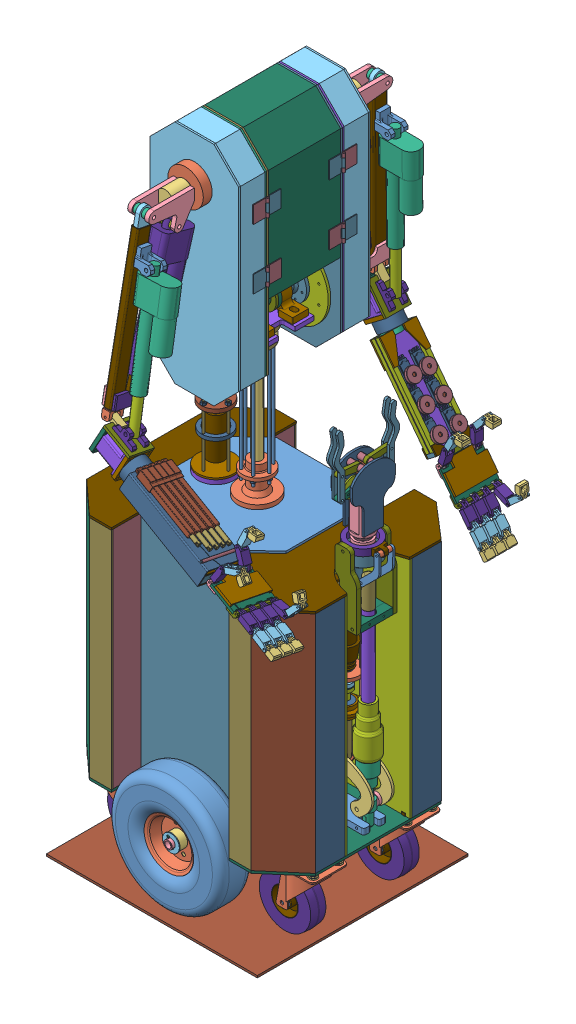
SolidWorks assembly sorbot, configuration По умолчанию. Lengths in mm. (continued)
Mates (geometry in assembly coordinates): (continued)
- Концентричный339: concentric aligned: cylinder of palm.fixture.p13-1 through (365.6621 758.5087 201.9382) axis (-0.001246 0.191494 0.981493) radius 1.5; cylinder of finger.p1-2 through (365.6602 758.8068 203.466) axis (-0.001246 0.191494 0.981493) radius 1.5
- Концентричный342: concentric aligned: cylinder of palm.fixture.p13-1 through (365.6621 758.5087 201.9382) axis (-0.001246 0.191494 0.981493) radius 1.5; cylinder of finger.p1-3 through (365.5966 768.573 253.5221) axis (-0.001246 0.191494 0.981493) radius 1.5
- Параллельность165: parallel aligned: plane of palm.p1-3 through (361.7576 760.7842 201.5469) normal (0.410922 0.894897 -0.174077); plane of finger.p1-3 through (409.4727 760.6234 276.0154) normal (0.410922 0.894897 -0.174077)
- Совпадение637: coincident anti-aligned: plane of palm.p1-3 through (359.2921 755.4149 202.5914) normal (-0.410922 -0.894897 0.174077); plane of palm.p3.m-1 through (320.3506 791.7274 297.3428) normal (0.410922 0.894897 -0.174077)
- Совпадение638: coincident aligned: plane of palm.p1-3 through (293.2577 810.1661 293.7109) normal (-0.001246 0.191494 0.981493); plane of palm.p3.m-1 through (294.9764 811.5594 293.4412) normal (-0.001246 0.191494 0.981493)
- Совпадение640: coincident anti-aligned: plane of palm.p3.m-1 through (303.6145 808.8356 293.9836) normal (0.91167 -0.4031 0.079805); plane of palm.p1-3 through (302.4043 801.5393 270.9531) normal (-0.91167 0.4031 -0.079805)
- Совпадение641: coincident anti-aligned: plane of palm.p3-1 through (354.922 753.9955 207.957) normal (-0.001246 0.191494 0.981493); plane of finger.p1-2 through (353.8618 756.4881 207.4694) normal (0.001246 -0.191494 -0.981493)
- Концентричный345: concentric aligned: cylinder of palm.fixture.p13-1 through (365.6621 758.5087 201.9382) axis (-0.001246 0.191494 0.981493) radius 1.5; cylinder of finger.p1-4 through (365.6284 763.6899 228.494) axis (-0.001246 0.191494 0.981493) radius 1.5
- Параллельность167: parallel aligned: plane of palm.p1-3 through (361.7576 760.7842 201.5469) normal (0.410922 0.894897 -0.174077); plane of finger.p1-4 through (409.5045 755.7403 250.9873) normal (0.410922 0.894897 -0.174077)
- Совпадение645: coincident anti-aligned: plane of palm.p1-3 through (359.2921 755.4149 202.5914) normal (-0.410922 -0.894897 0.174077); plane of palm.p3.m-2 through (320.4484 776.6951 220.2956) normal (0.410922 0.894897 -0.174077)
- Совпадение646: coincident aligned: plane of palm.p1-3 through (293.3824 791.0167 195.5616) normal (0.001246 -0.191494 -0.981493); plane of palm.p3.m-2 through (295.1011 792.41 195.2919) normal (0.001246 -0.191494 -0.981493)
- Совпадение647: coincident anti-aligned: plane of palm.p3.m-2 through (303.7123 793.8034 216.9364) normal (0.91167 -0.4031 0.079805); plane of palm.p1-3 through (302.4692 791.5816 219.9154) normal (-0.91167 0.4031 -0.079805)
- Заблокировать267: lock: unknown of ?; unknown of ?
- Концентричный348: concentric aligned: cylinder of palm.p3.m-1 through (297.351 805.9631 294.5361) axis (0.001246 -0.191494 -0.981493) radius 1.5; cylinder of finger.p1-5 through (297.3517 805.8673 294.0454) axis (0.001246 -0.191494 -0.981493) radius 1.5
- Совпадение648: coincident anti-aligned: plane of palm.p3.m-1 through (284.5507 802.4864 291.1227) normal (0.001246 -0.191494 -0.981493); plane of finger.p1-5 through (287.412 798.2914 291.9448) normal (-0.001246 0.191494 0.981493)
- Концентричный351: concentric aligned: cylinder of finger.p1-6 through (297.4494 790.8542 217.0963) axis (0.001246 -0.191494 -0.981493) radius 1.5; cylinder of palm.p3.m-2 through (297.4489 790.9308 217.4889) axis (0.001246 -0.191494 -0.981493) radius 1.5
- Концентричный352: concentric aligned: cylinder of finger.p1-1 through (402.282 756.6831 281.8693) axis (-0.001246 0.191494 0.981493) radius 1.5; cylinder of finger.p2-7 through (402.282 756.6831 281.8693) axis (-0.001246 0.191494 0.981493) radius 1.5
- Совпадение652: coincident anti-aligned: plane of finger.p1-1 through (393.5748 758.839 298.2487) normal (0.001246 -0.191494 -0.981493); plane of finger.p2-7 through (390.7532 760.3857 297.9434) normal (-0.001246 0.191494 0.981493)
- Концентричный354: concentric aligned: cylinder of finger.p3-1 through (437.4075 740.08 285.2682) axis (-0.001246 0.191494 0.981493) radius 1.5; cylinder of finger.p2-7 through (437.4076 740.0584 285.1575) axis (-0.001246 0.191494 0.981493) radius 1.5
- Совпадение653: coincident: plane of ? through (235.2448 521.1837 179.8569) normal (0.004463 0.000114 0.99999); plane of ? through (237.0318 518.7761 179.8492) normal (-0.004463 -0.000114 -0.99999)
- Концентричный355: concentric aligned: cylinder of finger.p1-3 through (402.3138 751.8 256.8412) axis (-0.001246 0.191494 0.981493) radius 1.5; cylinder of finger.p2-8 through (402.3138 751.8 256.8412) axis (-0.001246 0.191494 0.981493) radius 1.5
- Совпадение654: coincident anti-aligned: plane of finger.p1-3 through (393.6066 753.9559 273.2207) normal (0.001246 -0.191494 -0.981493); plane of finger.p2-8 through (390.7757 755.2583 272.963) normal (-0.001246 0.191494 0.981493)
- Концентричный356: concentric aligned: cylinder of finger.p1-4 through (402.3456 746.9169 231.8131) axis (-0.001246 0.191494 0.981493) radius 1.5; cylinder of finger.p2-9 through (402.3456 746.9169 231.8131) axis (-0.001246 0.191494 0.981493) radius 1.5
- Совпадение655: coincident anti-aligned: plane of finger.p1-4 through (393.6383 749.0728 248.1926) normal (0.001246 -0.191494 -0.981493); plane of finger.p2-9 through (390.8061 750.3187 247.9459) normal (-0.001246 0.191494 0.981493)
- Концентричный357: concentric aligned: cylinder of finger.p1-2 through (405.4877 751.586 204.9254) axis (-0.001246 0.191494 0.981493) radius 1.5; cylinder of finger.p2-10 through (405.4877 751.586 204.9254) axis (-0.001246 0.191494 0.981493) radius 1.5
- Совпадение656: coincident anti-aligned: plane of finger.p1-2 through (397.3122 751.6404 221.7155) normal (0.001246 -0.191494 -0.981493); plane of finger.p2-10 through (401.7717 744.0338 223.2052) normal (-0.001246 0.191494 0.981493)
- Концентричный358: concentric aligned: cylinder of finger.p3-2 through (431.4304 780.1948 199.4916) axis (-0.001246 0.191494 0.981493) radius 1.5; cylinder of finger.p2-10 through (431.4305 780.1732 199.3808) axis (-0.001246 0.191494 0.981493) radius 1.5
- Совпадение657: coincident anti-aligned: plane of finger.p3-2 through (439.6172 775.3981 217.134) normal (-0.001246 0.191494 0.981493); plane of finger.p2-10 through (429.781 774.8981 217.219) normal (0.001246 -0.191494 -0.981493)
- Концентричный359: concentric aligned: cylinder of finger.p1-5 through (317.4709 840.3743 287.3384) axis (0.001246 -0.191494 -0.981493) radius 1.5; cylinder of finger.p2-11 through (317.4709 840.3743 287.3384) axis (0.001246 -0.191494 -0.981493) radius 1.5
- Совпадение658: coincident anti-aligned: plane of finger.p1-5 through (309.7926 835.5044 284.2034) normal (0.001246 -0.191494 -0.981493); plane of finger.p2-11 through (306.0326 840.9226 283.1415) normal (-0.001246 0.191494 0.981493)
- Концентричный360: concentric aligned: cylinder of finger.p3-5 through (354.9027 851.1497 285.3986) axis (0.001246 -0.191494 -0.981493) radius 1.5; cylinder of finger.p2-11 through (354.9028 851.1281 285.2878) axis (0.001246 -0.191494 -0.981493) radius 1.5
- Совпадение659: coincident anti-aligned: plane of finger.p3-5 through (352.0131 861.3071 279.2228) normal (-0.001246 0.191494 0.981493); plane of finger.p2-11 through (346.4462 852.5329 280.9276) normal (0.001246 -0.191494 -0.981493)
- Концентричный362: concentric aligned: cylinder of finger.p1-6 through (278.3051 825.8821 210.2379) axis (0.001246 -0.191494 -0.981493) radius 1.5; cylinder of finger.p2-12 through (278.3051 825.8821 210.2379) axis (0.001246 -0.191494 -0.981493) radius 1.5
- Совпадение661: coincident anti-aligned: plane of finger.p1-6 through (277.7816 816.5471 207.9831) normal (0.001246 -0.191494 -0.981493); plane of finger.p2-12 through (270.3574 816.9317 207.8986) normal (-0.001246 0.191494 0.981493)
- Концентричный363: concentric aligned: cylinder of ? through (195.7839 707.1121 106.7239) axis (-0.004463 -0.000114 -0.99999) radius 1.5; cylinder of ? through (195.7834 707.1121 106.6111) axis (-0.004463 -0.000114 -0.99999) radius 1.5
- Совпадение662: coincident: plane of ? through (190.3026 717.2558 102.6343) normal (0.004463 0.000114 0.99999); plane of ? through (187.0589 706.2794 102.6501) normal (-0.004463 -0.000114 -0.99999)
- Совпадение664: coincident anti-aligned: plane of palm.p3-1 through (365.7816 761.5097 272.221) normal (0.001246 -0.191494 -0.981493); plane of finger.p1-3 through (353.3954 771.831 270.1915) normal (-0.001246 0.191494 0.981493)
- Совпадение665: coincident anti-aligned: plane of palm.p3-1 through (365.8134 756.6266 247.1929) normal (0.001246 -0.191494 -0.981493); plane of finger.p1-4 through (353.4271 766.9479 245.1634) normal (-0.001246 0.191494 0.981493)
- Совпадение666: coincident anti-aligned: plane of palm.p1-3 through (361.7576 760.7842 201.5469) normal (0.410922 0.894897 -0.174077); plane of palm.p5-1 through (331.4609 789.3117 276.6833) normal (-0.410922 -0.894897 0.174077)
- Совпадение667: coincident anti-aligned: plane of palm.p1-3 through (361.7576 760.7842 201.5469) normal (0.410922 0.894897 -0.174077); plane of palm.p6-1 through (302.9044 799.3879 261.0737) normal (-0.410922 -0.894897 0.174077)
- Совпадение668: coincident anti-aligned: plane of palm.p1-3 through (361.7576 760.7842 201.5469) normal (0.410922 0.894897 -0.174077); plane of palm.p5-2 through (331.5169 778.2186 219.7881) normal (-0.410922 -0.894897 0.174077)
- Совпадение669: coincident anti-aligned: plane of palm.p1-3 through (361.7576 760.7842 201.5469) normal (0.410922 0.894897 -0.174077); plane of palm.p6-2 through (302.8729 793.2734 229.5656) normal (-0.410922 -0.894897 0.174077)
- Заблокировать268: lock: unknown of ?; unknown of ?
- Заблокировать269: lock: unknown of ?; unknown of ?
- Концентричный367: concentric anti-aligned: cylinder of finger.actuator.p2-5 through (240.3211 845.5977 266.3536) axis (-0.91167 0.4031 -0.079805) radius 4.5; cylinder of finger.actuator.p1-3 through (128.7399 894.9339 256.5862) axis (0.91167 -0.4031 0.079805) radius 4.5
- Параллельность169: parallel anti-aligned: cylinder of finger.actuator.p1-3 through (90.9006 912.4285 257.2003) axis (0.001246 -0.191494 -0.981493) radius 2.1; cylinder of finger.actuator.p2-5 through (243.9733 843.1236 262.2561) axis (-0.001246 0.191494 0.981493) radius 2.1
- Концентричный368: concentric anti-aligned: cylinder of finger.actuator.p1-4 through (128.7773 889.1891 227.1414) axis (0.91167 -0.4031 0.079805) radius 4.5; cylinder of finger.actuator.p2-6 through (255.2287 833.2779 238.2105) axis (-0.91167 0.4031 -0.079805) radius 4.5
- Параллельность171: parallel anti-aligned: cylinder of finger.actuator.p1-4 through (90.938 906.6837 227.7555) axis (0.001246 -0.191494 -0.981493) radius 2.1; cylinder of finger.actuator.p2-6 through (258.881 830.8038 234.113) axis (-0.001246 0.191494 0.981493) radius 2.1
- Концентричный370: concentric anti-aligned: cylinder of finger.actuator.p1-5 through (128.7586 892.0615 241.8638) axis (0.91167 -0.4031 0.079805) radius 4.5; cylinder of finger.actuator.p2-7 through (254.035 836.6698 252.8301) axis (-0.91167 0.4031 -0.079805) radius 4.5
- Параллельность173: parallel anti-aligned: cylinder of finger.actuator.p1-5 through (90.9193 909.5561 242.4779) axis (0.001246 -0.191494 -0.981493) radius 2.1; cylinder of finger.actuator.p2-7 through (257.6873 834.1957 248.7326) axis (-0.001246 0.191494 0.981493) radius 2.1
- Концентричный371: concentric anti-aligned: cylinder of finger.actuator.p1-6 through (128.8147 883.4443 197.6966) axis (0.91167 -0.4031 0.079805) radius 4.5; cylinder of finger.actuator.p2-8 through (255.925 827.2418 208.8234) axis (-0.91167 0.4031 -0.079805) radius 4.5
- Параллельность175: parallel anti-aligned: cylinder of finger.actuator.p1-6 through (90.9754 900.9389 198.3107) axis (0.001246 -0.191494 -0.981493) radius 2.1; cylinder of finger.actuator.p2-8 through (259.5773 824.7676 204.7259) axis (-0.001246 0.191494 0.981493) radius 2.1
- Концентричный372: concentric anti-aligned: cylinder of finger.actuator.p1-7 through (128.796 886.3167 212.419) axis (0.91167 -0.4031 0.079805) radius 4.5; cylinder of ? through (255.6249 830.2386 223.5212) axis (-0.91167 0.4031 -0.079805) radius 4.5
- Параллельность177: parallel anti-aligned: cylinder of finger.actuator.p1-7 through (90.9567 903.8113 213.0331) axis (0.001246 -0.191494 -0.981493) radius 2.1; cylinder of ? through (259.2772 827.7644 219.4237) axis (-0.001246 0.191494 0.981493) radius 2.1
- Заблокировать270: lock: unknown of ?; unknown of ?
- Заблокировать271: lock: unknown of ?; unknown of ?
- Совпадение675: coincident anti-aligned: plane of arm.cap-1 through (83.1026 909.5205 266.9275) normal (0.410922 0.894897 -0.174077); plane of finger.actuator.p1-5 through (125.6674 886.786 250.5306) normal (-0.410922 -0.894897 0.174077)
- Совпадение676: coincident anti-aligned: plane of arm.cap-1 through (83.1026 909.5205 266.9275) normal (0.410922 0.894897 -0.174077); plane of finger.actuator.p1-7 through (125.7048 881.0411 221.0858) normal (-0.410922 -0.894897 0.174077)
- Совпадение677: coincident anti-aligned: plane of arm.cap-1 through (83.1026 909.5205 266.9275) normal (0.410922 0.894897 -0.174077); plane of finger.actuator.p1-4 through (125.6861 883.9136 235.8082) normal (-0.410922 -0.894897 0.174077)
- Совпадение678: coincident anti-aligned: plane of arm.cap-1 through (83.1026 909.5205 266.9275) normal (0.410922 0.894897 -0.174077); plane of finger.actuator.p1-6 through (125.7235 878.1687 206.3634) normal (-0.410922 -0.894897 0.174077)
- Заблокировать272: lock: unknown of ?; unknown of ?
- Заблокировать273: lock: unknown of ?; unknown of ?
- Заблокировать274: lock: unknown of ?; unknown of ?
- Концентричный373: concentric aligned: cylinder of finger.actuator.p1-3 through (90.9006 912.4285 257.2003) axis (0.001246 -0.191494 -0.981493) radius 2.1; cylinder of finger.actuator.p1-5 through (90.9193 909.5561 242.4779) axis (0.001246 -0.191494 -0.981493) radius 2.1
- Концентричный374: concentric aligned: cylinder of finger.actuator.p1-3 through (90.9006 912.4285 257.2003) axis (0.001246 -0.191494 -0.981493) radius 2.1; cylinder of finger.actuator.p1-4 through (90.938 906.6837 227.7555) axis (0.001246 -0.191494 -0.981493) radius 2.1
- Концентричный375: concentric aligned: cylinder of finger.actuator.p1-3 through (90.9006 912.4285 257.2003) axis (0.001246 -0.191494 -0.981493) radius 2.1; cylinder of finger.actuator.p1-7 through (90.9567 903.8113 213.0331) axis (0.001246 -0.191494 -0.981493) radius 2.1
- Концентричный376: concentric aligned: cylinder of finger.actuator.p1-3 through (90.9006 912.4285 257.2003) axis (0.001246 -0.191494 -0.981493) radius 2.1; cylinder of finger.actuator.p1-6 through (90.9754 900.9389 198.3107) axis (0.001246 -0.191494 -0.981493) radius 2.1
- Совпадение680: coincident anti-aligned: plane of finger.actuator.p1-3 through (131.8312 900.2094 247.9194) normal (0.001246 -0.191494 -0.981493); plane of finger.actuator.p1-5 through (131.8312 900.2094 247.9194) normal (-0.001246 0.191494 0.981493)
- Совпадение681: coincident anti-aligned: plane of finger.actuator.p1-4 through (131.8499 897.337 233.197) normal (-0.001246 0.191494 0.981493); plane of finger.actuator.p1-5 through (131.8499 897.337 233.197) normal (0.001246 -0.191494 -0.981493)
- Совпадение682: coincident anti-aligned: plane of finger.actuator.p1-4 through (131.8686 894.4646 218.4746) normal (0.001246 -0.191494 -0.981493); plane of finger.actuator.p1-7 through (131.8686 894.4646 218.4746) normal (-0.001246 0.191494 0.981493)
- Совпадение683: coincident anti-aligned: plane of finger.actuator.p1-6 through (131.8873 891.5922 203.7522) normal (-0.001246 0.191494 0.981493); plane of finger.actuator.p1-7 through (131.8873 891.5922 203.7522) normal (0.001246 -0.191494 -0.981493)
- Заблокировать275: lock: unknown of ?; unknown of ?
- Заблокировать276: lock: unknown of ?; unknown of ?
- Заблокировать277: lock: unknown of ?; unknown of ?
- Заблокировать278: lock: unknown of ?; unknown of ?
- Заблокировать279: lock: unknown of ?; unknown of ?
- Концентричный378: concentric aligned: cylinder of fingers.fixture.p2-2 through (272.0168 832.2235 287.0411) axis (0.001246 -0.191494 -0.981493) radius 2; cylinder of fingers.fixture.p1-2 through (272.014 832.6632 289.2946) axis (0.001246 -0.191494 -0.981493) radius 1.75
- Совпадение690: coincident anti-aligned: plane of lower.arm.p8-2 through (267.6618 778.8108 292.664) normal (0.91167 -0.4031 0.079805); plane of palm.fixture.p14-1 through (271.2358 781.1563 263.6829) normal (-0.91167 0.4031 -0.079805)
- Совпадение692: coincident anti-aligned: plane of arm.p1.m-1 through (-3.763 974.0415 223.4385) normal (1 0 0); plane of forearm.rotate.p12-m-1 through (-3.763 994.3192 220.6386) normal (-1 0 0)
- Параллельность178: parallel aligned: plane of forearm.rotate.p12-m-1 through (-3.763 974.256 224.5414) normal (0 0.190943 0.981601); plane of arm.p1.m-1 through (-18.263 974.7098 226.8741) normal (0 0.190943 0.981601)
- Заблокировать282: lock: unknown of ?; unknown of ?
- Совпадение696: coincident anti-aligned: plane of ? through (5.2041 922.3385 146.0785) normal (-0.840373 -0.541996 0.003813); plane of ? through (35.0967 876.1313 166.2278) normal (0.840373 0.541996 -0.003813)
- Заблокировать283: lock: unknown of ?; unknown of ?
- Заблокировать284: lock: unknown of ?; unknown of ?
- Заблокировать286: lock: unknown of ?; unknown of ?
- Концентричный381: concentric aligned: cylinder of finger.p3-3 through (437.7973 735.9485 260.107) axis (-0.001246 0.191494 0.981493) radius 1.5; cylinder of finger.p2-8 through (437.7975 735.9245 259.9837) axis (-0.001246 0.191494 0.981493) radius 1.5
- Концентричный382: concentric aligned: cylinder of finger.p3-4 through (437.9098 731.2007 234.8449) axis (-0.001246 0.191494 0.981493) radius 1.5; cylinder of finger.p2-9 through (437.9097 731.2157 234.9217) axis (-0.001246 0.191494 0.981493) radius 1.5
- Заблокировать287: lock: unknown of ?; unknown of ?
- Заблокировать288: lock: unknown of ?; unknown of ?
- Заблокировать289: lock: unknown of ?; unknown of ?
- Заблокировать290: lock: unknown of ?; unknown of ?
- Заблокировать291: lock: unknown of ?; unknown of ?
- Заблокировать293: lock: unknown of ?; unknown of ?
- Заблокировать294: lock: unknown of ?; unknown of ?
- Заблокировать295: lock: unknown of ?; unknown of ?
- Заблокировать296: lock: unknown of ?; unknown of ?
- Заблокировать297: lock: unknown of ?; unknown of ?
- Заблокировать298: lock: unknown of ?; unknown of ?
- Заблокировать299: lock: unknown of ?; unknown of ?
- Заблокировать301: lock: unknown of ?; unknown of ?
- Заблокировать302: lock: unknown of ?; unknown of ?
- Заблокировать304: lock: unknown of ?; unknown of ?
- Заблокировать305: lock: unknown of ?; unknown of ?
- Заблокировать306: lock: unknown of ?; unknown of ?
- Заблокировать307: lock: unknown of ?; unknown of ?
- Заблокировать308: lock: unknown of ?; unknown of ?
- Заблокировать309: lock: unknown of ?; unknown of ?
- Заблокировать310: lock: unknown of ?; unknown of ?
- Заблокировать311: lock: unknown of ?; unknown of ?
- Заблокировать313: lock: unknown of ?; unknown of ?
- Концентричный385: concentric aligned: cylinder of forearm.rotate.p9-1 through (-12.6985 951.7393 197.5021) axis (0 0.190943 0.981601) radius 2.5; cylinder of forearm.rotate.p10-1 through (-12.6985 953.4041 206.0607) axis (0 0.190943 0.981601) radius 2.5
- Заблокировать314: lock: unknown of ?; unknown of ?
- Заблокировать315: lock: unknown of ?; unknown of ?
- Заблокировать316: lock: unknown of ?; unknown of ?
- Заблокировать317: lock: unknown of ?; unknown of ?
- Заблокировать318: lock: unknown of ?; unknown of ?
- Совпадение698: coincident anti-aligned: plane of forearm.rotate.p7-1 through (65.0333 926.3354 250.3973) normal (0.410922 0.894897 -0.174077); plane of forearm.rotate.p8-1 through (58.959 925.2061 230.253) normal (-0.410922 -0.894897 0.174077)
- Совпадение699: coincident anti-aligned: plane of forearm.rotate.p7-1 through (65.0333 926.3354 250.3973) normal (0.410922 0.894897 -0.174077); plane of forearm.rotate.p8-2 through (58.959 919.4778 200.805) normal (-0.410922 -0.894897 0.174077)
- Заблокировать319: lock: unknown of ?; unknown of ?
- Концентричный386: concentric aligned: cylinder of body.frame.p1-3 through (-12.4559 1335.4922 -50.7442) axis (0 0 1) radius 43; cylinder of arm.fixture.cap-1 through (-12.4559 1335.4922 -73.2442) axis (0 0 1) radius 45
- Заблокировать330: lock: unknown of ?; unknown of ?
- Заблокировать336: lock: unknown of ?; unknown of ?
- Заблокировать337: lock: unknown of ?; unknown of ?
- Заблокировать344: lock: unknown of body_tilt_drive_frame_cap-1; unknown of ?
- Заблокировать351: lock: unknown of turret.table.cap-1; unknown of body_tilt_drive_frame_cap-1
- Совпадение740: coincident anti-aligned: plane of shoulder.bearing.housing-2 through (-12.4903 1335.516 -46.7442) normal (0 0 1); plane of body.frame.p4.right-1 through (-117.4903 1436.2936 -46.7442) normal (0 0 -1)
- Концентричный404: concentric aligned: cylinder of shoulder.bearing.housing-1 through (-12.7629 1335.3853 40.2558) axis (0 0 -1) radius 15.5; cylinder of ? through (-12.7629 1335.3853 44.2558) axis (0 0 -1) radius 15
- Совпадение742: coincident: unknown of ?; unknown of ?
- Заблокировать361: lock: unknown of ?; unknown of ?
- Заблокировать362: lock: unknown of ?; unknown of ?
- Совпадение745: coincident anti-aligned: plane of body.frame.p5-1 through (92.4017 957.5916 592.5032) normal (1 0 0); plane of cap-hinge-1 through (92.4017 1325.4557 -46.5922) normal (-1 0 0)
- Совпадение746: coincident anti-aligned: plane of body.frame.p5-1 through (92.4017 957.5916 592.5032) normal (1 0 0); plane of cap-hinge-p1-2 through (92.4017 1182.6154 -46.8053) normal (-1 0 0)
- Концентричный405: concentric anti-aligned: cylinder of cap-hinge-2 through (95.4017 1143.4534 -46.8053) axis (0 1 0) radius 2; cylinder of cap-hinge-p1-2 through (95.4017 1182.6154 -46.8053) axis (0 -1 0) radius 2
- Совпадение747: coincident anti-aligned: plane of cap-hinge-2 through (75.4017 1173.4534 -40.9717) normal (0 -1 0); plane of cap-hinge-p1-2 through (75.4017 1173.4534 -41.8622) normal (0 1 0)
- Заблокировать363: lock: unknown of ?; unknown of ?
- Заблокировать364: lock: unknown of ?; unknown of ?
- Заблокировать365: lock: unknown of ?; unknown of ?
- Касательный31: tangent anti-aligned: cylinder of arm.actuator.p2-2 through (-12.7848 966.8747 173.3183) axis (0 0.960187 -0.279359) radius 10; plane of forearm.rotate.p12-1 through (-22.7848 1003.1156 189.6023) normal (1 0 0)
- Параллельность188: parallel anti-aligned: cylinder of arm.actuator-2/arm.actuator.p1-1 through (-27.7848 1286.6873 80.2712) axis (1 0 0) radius 4.1; cylinder of arm.actuator.p2-2 through (12.2152 975.0363 170.9438) axis (-1 0 0) radius 4
- Заблокировать368: lock: unknown of ?; unknown of ?
- Заблокировать369: lock: unknown of ?; unknown of ?
- Совпадение765: coincident anti-aligned: plane of arm.p1.m-1 through (-18.263 968.886 196.9353) normal (0 0.190943 0.981601); plane of shoulder.lever-1 through (-17.763 1332.6644 126.1724) normal (0 -0.190943 -0.981601)
- Концентричный406: concentric anti-aligned: cylinder of ? through (-27.7629 1335.3853 140.1602) axis (-1 0 0) radius 4; cylinder of shoulder.lever-1 through (-17.763 1335.3853 140.1602) axis (1 0 0) radius 4
- Концентричный408: concentric aligned: cylinder of ? through (-17.763 1335.3853 140.1602) axis (-1 0 0) radius 4; cylinder of ? through (-27.7629 1335.3853 140.1602) axis (-1 0 0) radius 4
- Совпадение757: coincident anti-aligned: plane of shoulder.lever-1 through (-17.763 1335.3854 140.1608) normal (-1 0 0); plane of ? through (-17.763 1335.3853 140.1602) normal (1 0 0)
- Концентричный409: concentric anti-aligned: cylinder of arm.actuator-2/arm.actuator.p1-1 through (-27.7848 1286.6873 80.2712) axis (1 0 0) radius 4.1; cylinder of ? through (-27.7629 1286.6873 80.2712) axis (-1 0 0) radius 4
- Совпадение759: coincident anti-aligned: plane of ? through (-27.7629 1335.3734 139.2441) normal (1 0 0); plane of ? through (-27.7629 1286.6873 80.2712) normal (-1 0 0)
- Концентричный411: concentric anti-aligned: cylinder of arm.actuator-2/arm.actuator.p1-1 through (-27.7848 1286.6873 80.2712) axis (1 0 0) radius 4.1; cylinder of ? through (-22.7629 1286.6873 80.2712) axis (-1 0 0) radius 4
- Совпадение760: coincident anti-aligned: plane of ? through (2.2371 1356.1502 -67.7442) normal (1 0 0); plane of ? through (2.2371 1335.3734 139.2441) normal (-1 0 0)
- Концентричный412: concentric anti-aligned: cylinder of shoulder.lever-1 through (-17.763 1335.3853 140.1602) axis (1 0 0) radius 4; cylinder of ? through (12.2371 1335.3853 140.1602) axis (-1 0 0) radius 4
- Концентричный413: concentric aligned: cylinder of ? through (12.2371 1335.3853 140.1602) axis (-1 0 0) radius 4; cylinder of ? through (2.2371 1335.3853 140.1602) axis (-1 0 0) radius 4
- Совпадение761: coincident anti-aligned: plane of ? through (2.2371 1335.3734 139.2441) normal (-1 0 0); plane of ? through (2.2371 1335.3853 140.1602) normal (1 0 0)
- Концентричный414: concentric anti-aligned: cylinder of arm.actuator-2/arm.actuator.p1-1 through (-27.7848 1286.6873 80.2712) axis (1 0 0) radius 4.1; cylinder of ? through (2.2371 1286.6873 80.2712) axis (-1 0 0) radius 4
- Совпадение762: coincident anti-aligned: plane of ? through (2.2371 1335.3734 139.2441) normal (-1 0 0); plane of ? through (2.2371 1286.6873 80.2712) normal (1 0 0)
- Концентричный416: concentric anti-aligned: cylinder of arm.actuator-2/arm.actuator.p1-1 through (-27.7848 1286.6873 80.2712) axis (1 0 0) radius 4.1; cylinder of ? through (12.2371 1286.6873 80.2712) axis (-1 0 0) radius 4
- Заблокировать370: lock: unknown of ?; unknown of ?
- Концентричный420: concentric aligned: cylinder of body.center-1 through (-20.0648 982.0246 -136.9555) axis (0 -1 0) radius 11; cylinder of ? through (-20.0648 982.0246 -136.9555) axis (0 -1 0) radius 11
- Заблокировать371: lock: unknown of body.center-1; unknown of body_pivot_fixture-1
- Совпадение768: coincident anti-aligned: plane of body_pivot_fixture-1 through (-20.0648 972.0246 -136.9555) normal (0 1 0); plane of ? through (-63.8424 972.0246 -151.4602) normal (0 -1 0)
- Заблокировать372: lock: unknown of ?; unknown of ?
- Концентричный421: concentric anti-aligned: cylinder of body_axis-1 through (-20.0648 1016.5246 -50.7475) axis (0 0 -1) radius 10.9; cylinder of ? through (-20.0648 1016.5246 -110.5942) axis (0 0 1) radius 11
- Совпадение776: coincident anti-aligned: plane of ? through (-63.8424 982.0246 -151.4602) normal (0 1 0); plane of ? through (1.9352 982.0246 -116.0942) normal (0 -1 0)
- Концентричный422: concentric aligned: cylinder of body_axis-1 through (-20.0648 1016.5246 -50.7475) axis (0 0 -1) radius 10.9; cylinder of ? through (-20.0648 1016.5246 -163.4875) axis (0 0 -1) radius 11
- Совпадение779: coincident anti-aligned: plane of ? through (-63.8424 982.0246 -151.4602) normal (0 1 0); plane of ? through (1.9352 982.0246 -157.9875) normal (0 -1 0)
- Совпадение783: coincident aligned: plane of body_tilt_drive_frame_cap-1 through (-173.1373 715.2934 -206.9448) normal (0 0 -1); plane of body_tilt_drive_frame_p6-3 through (-171.1373 1083.0403 -206.9448) normal (0 0 -1)
- Концентричный430: concentric anti-aligned: cylinder of tilt.thread.rod-1 through (-118.5699 948.5591 -137.5376) axis (0 -1 0) radius 8; cylinder of tilt.thread.rod.fixture.2-1 through (-118.5699 794.5591 -137.5376) axis (0 1 0) radius 8
- Совпадение797: coincident anti-aligned: plane of tilt.thread.rod-1 through (-118.5699 794.5591 -137.5376) normal (0 -1 0); plane of tilt.thread.rod.fixture.2-1 through (-118.5699 794.5591 -137.5376) normal (0 1 0)
- Концентричный431: concentric: cylinder of tilt.thread.rod-1 through (-118.5699 947.5591 -137.5376) axis (0 -1 0) radius 8; cylinder of tilit.thread.rod.bearing.fixture-1 through (-118.5701 937.0246 -137.4966) axis (0 -1 0) radius 6.5
- Совпадение799: coincident anti-aligned: plane of tilit.thread.rod.bearing.fixture-1 through (-20.0648 937.0246 -136.9555) normal (0 1 0); plane of ? through (-118.5699 937.0246 -137.5376) normal (0 -1 0)
- Концентричный432: concentric anti-aligned: cylinder of tilt.thread.rod-1 through (-118.5699 928.5591 -137.5376) axis (0 1 0) radius 6; cylinder of ? through (-118.5699 945.0246 -137.5376) axis (0 -1 0) radius 6
- Совпадение800: coincident anti-aligned: plane of tilit.thread.rod.bearing.fixture-1 through (-20.0648 937.0246 -136.9555) normal (0 1 0); plane of ? through (-118.5699 937.0246 -137.5376) normal (0 -1 0)
- Концентричный433: concentric aligned: cylinder of ? through (-118.5699 945.0246 -137.5376) axis (0 -1 0) radius 14; cylinder of ? through (-118.5699 945.0246 -137.5376) axis (0 -1 0) radius 14
- Концентричный434: concentric anti-aligned: cylinder of body_axis-1 through (-20.0648 1016.5246 -50.7475) axis (0 0 -1) radius 10.9; cylinder of body_tilt_axis_clamp-1 through (-20.0648 1016.5246 -155.4875) axis (0 0 1) radius 11
- Совпадение801: coincident anti-aligned: plane of ? through (-20.0648 1016.5246 -163.4875) normal (0 0 1); plane of body_tilt_axis_clamp-1 through (-20.0648 1016.5246 -163.4875) normal (0 0 -1)
- Концентричный435: concentric aligned: cylinder of body_axis-1 through (-20.0648 1016.5246 -50.7475) axis (0 0 -1) radius 10.9; cylinder of body_tilt_axis_clamp-2 through (-20.0648 1016.5246 -110.5942) axis (0 0 -1) radius 10.9
- Совпадение802: coincident anti-aligned: plane of ? through (-20.0648 1016.5246 -110.5942) normal (0 0 -1); plane of body_tilt_axis_clamp-2 through (-20.0648 1016.5246 -110.5942) normal (0 0 1)
- Концентричный436: concentric anti-aligned: cylinder of body_tilt_axis_clamp-1 through (-20.0648 1016.5246 -155.4875) axis (0 0 1) radius 20; cylinder of body_tilt_lever-1 through (-20.0648 1016.5246 -149.4875) axis (0 0 -1) radius 20
- Совпадение803: coincident anti-aligned: plane of body_tilt_axis_clamp-1 through (-20.0648 1016.5246 -155.4875) normal (0 0 1); plane of body_tilt_lever-1 through (-97.2168 978.7734 -155.4875) normal (0 0 -1)
- Заблокировать382: lock: unknown of ?; unknown of ?
- Заблокировать383: lock: unknown of ?; unknown of ?
- Заблокировать386: lock: unknown of ?; unknown of ?
- Заблокировать387: lock: unknown of ?; unknown of ?
- Заблокировать388: lock: unknown of body_pivot_fixture-1; unknown of body_pivot-2
- Заблокировать389: lock: unknown of ?; unknown of ?
- Заблокировать391: lock: unknown of body_pivot_fixture-1; unknown of ?
- Концентричный439: concentric aligned: cylinder of body_tilt_axis_clamp-2 through (-20.0648 1016.5246 -118.5942) axis (0 0 -1) radius 20; cylinder of body_tilt_lever-2 through (-20.0648 1016.5246 -118.5942) axis (0 0 -1) radius 20
- Концентричный440: concentric aligned: cylinder of body_tilt_lever-1 through (-99.3474 976.856 -149.4875) axis (0 0 -1) radius 5; cylinder of body_tilt_lever-2 through (-99.3474 976.856 -118.5942) axis (0 0 -1) radius 5
- Совпадение805: coincident anti-aligned: plane of body_tilt_axis_clamp-2 through (-20.0648 1016.5246 -118.5942) normal (0 0 -1); plane of body_tilt_lever-2 through (-97.2168 978.7734 -118.5942) normal (0 0 1)
- Концентричный441: concentric aligned: cylinder of body_tilt_lever-1 through (-99.3474 976.856 -149.4875) axis (0 0 -1) radius 5; cylinder of body_tilt_lever_axis-1 through (-99.3474 976.856 -80.4875) axis (0 0 -1) radius 5
- Расстояние22: distance = 40 mm aligned: plane of body_tilt_lever-1 through (-97.2168 978.7734 -155.4875) normal (0 0 -1); plane of body_tilt_lever_axis-1 through (-99.3474 976.856 -195.4875) normal (0 0 -1)
- Концентричный442: concentric anti-aligned: cylinder of body.tilit.lever.2-1 through (-99.3474 976.856 -184.3819) axis (0 0 1) radius 5; cylinder of body_tilt_lever_axis-1 through (-99.3474 976.856 -80.4875) axis (0 0 -1) radius 5
- Концентричный443: concentric anti-aligned: cylinder of tilt.thread.rod-1 through (-118.5699 928.5591 -137.5376) axis (0 1 0) radius 6; cylinder of body.tilt.nut-1 through (-118.5699 842.2928 -137.5376) axis (0 -1 0) radius 8
- Концентричный444: concentric anti-aligned: cylinder of tilt.thread.rod-1 through (-118.5699 928.5591 -137.5376) axis (0 1 0) radius 6; cylinder of body.tilit.nut.housing-1 through (-118.5699 838.2928 -137.5376) axis (0 -1 0) radius 8
- Концентричный445: concentric anti-aligned: cylinder of body.tilit.lever.2-1 through (-118.5699 828.2928 -184.3819) axis (0 0 1) radius 5; cylinder of body.tilit.nut.housing-1 through (-118.5699 828.2928 -152.3819) axis (0 0 -1) radius 5
- Концентричный446: concentric aligned: cylinder of body.tilit.nut.housing-1 through (-118.5699 828.2928 -152.3819) axis (0 0 -1) radius 5; cylinder of body.tilit.nut.housing.bolt-1 through (-118.5699 828.2928 -154.3819) axis (0 0 -1) radius 5
- Совпадение808: coincident anti-aligned: plane of body.tilt.nut-1 through (-109.5699 828.2928 -121.9491) normal (0 -1 0); plane of body.tilit.nut.housing-1 through (-93.5699 828.2928 -153.1376) normal (0 1 0)
- Параллельность198: parallel anti-aligned: plane of body.tilt.nut-1 through (-109.5699 842.2928 -153.126) normal (0 0 -1); plane of body.tilit.nut.housing-1 through (-143.5699 828.2928 -153.1376) normal (0 0 1)
- Заблокировать392: lock: unknown of ?; unknown of ?
- Совпадение810: coincident anti-aligned: plane of body.tilit.lever.2-1 through (-118.5699 828.2928 -177.3819) normal (0 0 1); plane of body.tilit.nut.housing-1 through (-140.5568 838.2928 -177.3819) normal (0 0 -1)
- Совпадение811: coincident anti-aligned: plane of body.tilit.lever.2-1 through (-118.5699 828.2928 -184.3819) normal (0 0 -1); plane of body.tilit.nut.housing.bolt-1 through (-128.835 829.9135 -184.3819) normal (0 0 1)
- Концентричный447: concentric anti-aligned: cylinder of body_tilt_lever_axis-1 through (-99.3474 976.856 -80.4875) axis (0 0 -1) radius 5; cylinder of body.tilit.extender-1 through (-99.3474 976.856 -176.9875) axis (0 0 1) radius 5
- Совпадение812: coincident anti-aligned: plane of body_tilt_lever-1 through (-97.2168 978.7734 -155.4875) normal (0 0 -1); plane of body.tilit.extender-1 through (-99.3474 976.856 -155.4875) normal (0 0 1)
- Концентричный448: concentric aligned: cylinder of body_tilt_lever_axis-1 through (-99.3474 976.856 -80.4875) axis (0 0 -1) radius 5; cylinder of washer-1 through (-99.3474 976.856 -184.3819) axis (0 0 -1) radius 5
- Совпадение813: coincident anti-aligned: plane of body.tilit.lever.2-1 through (-118.5699 828.2928 -184.3819) normal (0 0 -1); plane of washer-1 through (-99.3474 976.856 -184.3819) normal (0 0 1)
- Концентричный449: concentric anti-aligned: cylinder of body_tilt_lever_axis-1 through (-99.3474 976.856 -80.4875) axis (0 0 -1) radius 5; cylinder of body.tilit.extender-2 through (-99.3474 976.856 -118.5942) axis (0 0 1) radius 5
- Совпадение814: coincident anti-aligned: plane of body_tilt_lever-2 through (-97.2168 978.7734 -118.5942) normal (0 0 1); plane of body.tilit.extender-2 through (-99.3474 976.856 -118.5942) normal (0 0 -1)
- Концентричный450: concentric anti-aligned: cylinder of body_tilt_lever_axis-1 through (-99.3474 976.856 -80.4875) axis (0 0 -1) radius 5; cylinder of body.tilit.lever.2-2 through (-99.3474 976.856 -97.6932) axis (0 0 1) radius 5
- Концентричный451: concentric aligned: cylinder of body.tilit.nut.housing-1 through (-118.5699 828.2928 -122.6932) axis (0 0 1) radius 5; cylinder of body.tilit.lever.2-2 through (-118.5699 828.2928 -97.6932) axis (0 0 1) radius 5
- Совпадение816: coincident anti-aligned: plane of body.tilit.nut.housing-1 through (-140.5568 838.2928 -97.6932) normal (0 0 1); plane of body.tilit.lever.2-2 through (-118.5699 828.2928 -97.6932) normal (0 0 -1)
- Концентричный452: concentric aligned: cylinder of body.tilit.nut.housing-1 through (-118.5699 828.2928 -122.6932) axis (0 0 1) radius 5; cylinder of body.tilit.nut.housing.bolt-2 through (-118.5699 828.2928 -120.6932) axis (0 0 1) radius 5
- Совпадение817: coincident anti-aligned: plane of body.tilit.lever.2-2 through (-118.5699 828.2928 -90.6932) normal (0 0 1); plane of body.tilit.nut.housing.bolt-2 through (-108.3047 829.9135 -90.6932) normal (0 0 -1)
- Концентричный453: concentric aligned: cylinder of body_tilt_lever_axis-1 through (-99.3474 976.856 -80.4875) axis (0 0 -1) radius 5; cylinder of washer-2 through (-99.3474 976.856 -88.6932) axis (0 0 -1) radius 5
- Совпадение818: coincident anti-aligned: plane of body.tilit.lever.2-2 through (-118.5699 828.2928 -90.6932) normal (0 0 1); plane of washer-2 through (-99.3474 976.856 -90.6932) normal (0 0 -1)
- Совпадение819: coincident anti-aligned: plane of body.frame.p1-3 through (92.5097 1436.2936 -50.7442) normal (0 0 -1); plane of arm.fixture.cap-1 through (-12.4559 1335.4922 -50.7442) normal (0 0 1)
- Совпадение820: coincident anti-aligned: plane of finger.p3-2 through (439.6172 775.3981 217.134) normal (-0.001246 0.191494 0.981493); plane of finger.p2-10 through (429.781 774.8981 217.219) normal (0.001246 -0.191494 -0.981493)
- Заблокировать394: lock: unknown of ?; unknown of ?
- Заблокировать395: lock: unknown of ?; unknown of ?
- Заблокировать396: lock: unknown of ?; unknown of ?
- Заблокировать397: lock: unknown of ?; unknown of ?
- Заблокировать398: lock: unknown of ?; unknown of ?
- Заблокировать399: lock: unknown of ?; unknown of ?
- Заблокировать402: lock: unknown of ?; unknown of ?
- Заблокировать405: lock: unknown of ?; unknown of ?
- Концентричный459: concentric anti-aligned: cylinder of cap-hinge-p1-3 through (95.5097 1327.1115 -226.3787) axis (0 -1 0) radius 2; cylinder of cap-hinge-5 through (95.5097 1287.9494 -226.3787) axis (0 1 0) radius 2
- Совпадение845: coincident anti-aligned: plane of cap-hinge-p1-3 through (75.5097 1317.9494 -221.4356) normal (0 1 0); plane of cap-hinge-5 through (75.5404 1317.9494 -220.4411) normal (0 -1 0)
- Заблокировать404: lock: unknown of ?; unknown of ?
- Заблокировать406: lock: unknown of ?; unknown of ?
- Концентричный460: concentric anti-aligned: cylinder of cap-hinge-p1-4 through (95.5097 1143.936 -226.3787) axis (0 1 0) radius 2; cylinder of cap-hinge-4 through (95.5097 1183.1735 -226.3787) axis (0 -1 0) radius 2
- Совпадение847: coincident anti-aligned: plane of cap-hinge-4 through (75.5097 1173.1735 -232.2123) normal (0 -1 0); plane of cap-hinge-p1-4 through (75.4842 1173.1735 -231.2174) normal (0 1 0)
- Заблокировать407: lock: unknown of ?; unknown of ?
- Заблокировать410: lock: unknown of ?; unknown of ?
- Совпадение849: coincident anti-aligned: plane of body_pivot_fixture-1 through (-20.0648 937.0246 -136.9555) normal (0 -1 0); plane of tilit.thread.rod.bearing.fixture-1 through (-20.0648 937.0246 -136.9555) normal (0 1 0)
- Заблокировать411: lock: unknown of body_pivot_fixture-1; unknown of ?
- Параллельность199: parallel aligned: plane of wall6-3 through (267.1742 -18.2461 -216.2424) normal (1 0 0); plane of ? through (92.0581 957.5993 348.483) normal (1 0 0)
- Заблокировать412: lock: unknown of ?; unknown of ?
- Совпадение851: coincident anti-aligned: plane of body.frame.p4-4 through (-117.3772 1436.2936 -226.3595) normal (0 0 1); plane of shoulder.bearing.housing-4 through (-12.3772 1335.516 -226.3595) normal (0 0 -1)
- Концентричный462: concentric aligned: cylinder of body.frame.p4-4 through (-12.3772 1335.516 -226.3595) axis (0 0 -1) radius 12.5; cylinder of shoulder.bearing.housing-4 through (-12.3772 1335.516 -205.3595) axis (0 0 -1) radius 15.5
- Заблокировать413: lock: unknown of ?; unknown of ?
- Концентричный463: concentric aligned: cylinder of shoulder.bearing.housing-3 through (-12.6499 1335.3853 -313.3595) axis (0 0 1) radius 15.5; cylinder of shoulder.axis-2 through (-12.6499 1335.3853 -317.3595) axis (0 0 1) radius 15
- Совпадение853: coincident aligned: plane of shoulder.bearing.housing-4 through (-12.3772 1335.516 -205.3595) normal (0 0 1); plane of shoulder.axis-2 through (-12.6499 1335.3853 -205.3595) normal (0 0 1)
- Совпадение855: coincident: plane of body.frame.p4-4 through (-117.3772 1436.2936 -230.3595) normal (0 0 -1); unknown of ?
- Совпадение856: coincident anti-aligned: plane of shoulder.p6-4 through (-12.6499 1335.3853 -288.3595) normal (0 0 -1); plane of body.frame.p4.external-1 through (-117.6384 1436.1749 -288.3595) normal (0 0 1)
- Концентричный464: concentric aligned: cylinder of shoulder.axis-2 through (-12.6499 1335.3853 -317.3595) axis (0 0 1) radius 15; cylinder of shoulder.p6-3 through (-12.6499 1335.3853 -245.2739) axis (0 0 1) radius 15
- Концентричный465: concentric anti-aligned: cylinder of shoulder.axis-2 through (-12.6499 1335.3853 -317.3595) axis (0 0 1) radius 15; cylinder of shoulder.p6-4 through (-12.6499 1335.3853 -270.3595) axis (0 0 -1) radius 15
- Совпадение857: coincident: unknown of ?; plane of shoulder.p4-3 through (-59.8188 1400.1357 -245.3595) normal (0 0 1)
- Совпадение858: coincident: plane of shoulder.p6-4 through (-12.6499 1335.3853 -270.3595) normal (0 0 1); plane of shoulder.p4-4 through (-59.8188 1400.1357 -276.3595) normal (0 0 -1)
- Концентричный466: concentric anti-aligned: cylinder of shoulder.axis-2 through (-12.6499 1335.3853 -317.3595) axis (0 0 1) radius 15; cylinder of shoulder.p4-4 through (-12.6499 1335.3853 -272.3595) axis (0 0 -1) radius 15
- Концентричный467: concentric anti-aligned: cylinder of shoulder.axis-2 through (-12.6499 1335.3853 -317.3595) axis (0 0 1) radius 15; cylinder of shoulder.p4-3 through (-12.6499 1335.3853 -245.3595) axis (0 0 -1) radius 15
- Совпадение865: coincident anti-aligned: plane of body.frame.p4-4 through (-117.3772 1436.2936 -230.3595) normal (0 0 -1); plane of arm.lift.actuator.fixture.p3-3 through (-88.5702 993.1387 -230.3595) normal (0 0 1)
- Концентричный469: concentric aligned: cylinder of arm.lift.actuator.fixture.p3-3 through (-88.5702 993.1387 -230.3595) axis (0 0 -1) radius 4; cylinder of arm.lift.actuator.fixture.p2-2 through (-88.5702 993.1387 -230.3595) axis (0 0 -1) radius 4
- Заблокировать416: lock: unknown of ?; unknown of ?
- Заблокировать415: lock: unknown of ?; unknown of ?
- Концентричный470: concentric anti-aligned: cylinder of arm.lift.actuator.fixture.p3-4 through (-88.5702 993.1387 -288.3595) axis (0 0 1) radius 4; cylinder of arm.lift.actuator.fixture.p2-2 through (-88.5702 993.1387 -230.3595) axis (0 0 -1) radius 4
- Концентричный478: concentric aligned: cylinder of arm.lift.actuator.fixture.p2-2 through (-88.5702 993.1387 -230.3595) axis (0 0 -1) radius 4; cylinder of arm.actuator-4/arm.actuator.p1-1 through (-88.5702 993.1387 -244.3595) axis (0 0 -1) radius 4.1
- Касательный33: tangent anti-aligned: plane of arm.lift.actuator.fixture.p3-3 through (-88.5702 993.1387 -249.3595) normal (0 0 -1); cylinder of arm.actuator-4/arm.actuator.p1-1 through (-89.1112 985.157 -259.3595) axis (0.067628 0.997711 0) radius 10
- Концентричный480: concentric anti-aligned: cylinder of arm.actuator-4/arm.actuator.p1-1 through (-79.508 1126.8319 -259.3595) axis (0.067628 0.997711 0) radius 10; cylinder of arm.actuator.p2-4 through (-60.3086 1410.0778 -259.3595) axis (-0.067628 -0.997711 0) radius 10
- Концентричный481: concentric anti-aligned: cylinder of shoulder.p4-3 through (-60.8835 1401.5972 -245.3595) axis (0 0 -1) radius 4; cylinder of arm.actuator.p2-4 through (-60.8835 1401.5972 -284.3595) axis (0 0 1) radius 4
- Концентричный482: concentric anti-aligned: cylinder of shoulder.p4-4 through (-60.8835 1401.5972 -272.3595) axis (0 0 -1) radius 4; cylinder of arm.actuator.p2-4 through (-60.8835 1401.5972 -284.3595) axis (0 0 1) radius 4
- Заблокировать418: lock: unknown of ?; unknown of ?
- Заблокировать419: lock: unknown of ?; unknown of ?
- Концентричный483: concentric anti-aligned: cylinder of arm.fixture-4 through (2.8485 1335.3868 -413.2628) axis (0.999986 0 0.005196) radius 4; cylinder of arm.lift2.actuator.fixture.p1-4 through (2.8485 1335.3868 -413.2628) axis (-0.999986 0 -0.005196) radius 4
- Совпадение869: coincident anti-aligned: plane of arm.fixture-4 through (2.8437 1335.375 -412.3468) normal (-0.999986 0 -0.005196); plane of arm.lift2.actuator.fixture.p1-4 through (2.8485 1335.3868 -413.2628) normal (0.999986 0 0.005196)
- Заблокировать420: lock: unknown of ?; unknown of ?
- Концентричный484: concentric aligned: cylinder of shoulder.lever-2 through (-7.1514 1335.3868 -413.3148) axis (-0.999986 0 -0.005196) radius 4; cylinder of arm.lift2.actuator.fixture.p1-4 through (2.8485 1335.3868 -413.2628) axis (-0.999986 0 -0.005196) radius 4
- Совпадение870: coincident anti-aligned: plane of shoulder.lever-2 through (-7.1514 1335.3868 -413.3154) normal (0.999986 0 0.005196); plane of arm.lift2.actuator.fixture.p1-4 through (-7.1514 1335.3868 -413.3148) normal (-0.999986 0 -0.005196)
- Концентричный485: concentric anti-aligned: cylinder of arm.fixture-5 through (-37.1514 1335.3868 -413.3148) axis (0.999986 0 0.005196) radius 4; cylinder of arm.lift2.actuator.fixture.p1-5 through (-17.1517 1335.3868 -413.2109) axis (-0.999986 0 -0.005196) radius 4
- Совпадение871: coincident anti-aligned: plane of arm.fixture-5 through (-27.1563 1335.375 -412.3468) normal (0.999986 0 0.005196); plane of arm.lift2.actuator.fixture.p1-5 through (-27.1515 1335.3868 -413.2628) normal (-0.999986 0 -0.005196)
- Заблокировать422: lock: unknown of ?; unknown of ?
- Концентричный486: concentric anti-aligned: cylinder of arm.fixture-4 through (2.5373 1286.6879 -353.3754) axis (0.999986 0 0.005196) radius 4; cylinder of arm.actuator-5/arm.actuator.p1-1 through (2.5373 1286.6879 -353.3754) axis (-0.999986 0 -0.005196) radius 4.1
- Концентричный487: concentric anti-aligned: cylinder of arm.fixture-4 through (2.5373 1286.6879 -353.3754) axis (0.999986 0 0.005196) radius 4; cylinder of arm.lift2.actuator.fixture.p1.m1-3 through (2.5373 1286.6879 -353.3754) axis (-0.999986 0 -0.005196) radius 4
- Совпадение873: coincident anti-aligned: plane of arm.fixture-4 through (2.8437 1335.375 -412.3468) normal (-0.999986 0 -0.005196); plane of arm.lift2.actuator.fixture.p1.m1-3 through (2.5373 1286.6879 -353.3754) normal (0.999986 0 0.005196)
- Концентричный488: concentric anti-aligned: cylinder of arm.fixture-5 through (-37.4626 1286.6879 -353.4274) axis (0.999986 0 0.005196) radius 4; cylinder of arm.lift2.actuator.fixture.p1.m1-4 through (-22.4628 1286.6879 -353.3495) axis (-0.999986 0 -0.005196) radius 4
- Совпадение874: coincident anti-aligned: plane of arm.fixture-5 through (-27.1563 1335.375 -412.3468) normal (0.999986 0 0.005196); plane of arm.lift2.actuator.fixture.p1.m1-4 through (-27.4627 1286.6879 -353.3754) normal (-0.999986 0 -0.005196)
- Касательный34: tangent anti-aligned: cylinder of arm.actuator-5/arm.actuator.p1-1 through (-12.4662 1294.6562 -352.7424) axis (0.000462 -0.996043 -0.088876) radius 10; plane of arm.lift2.actuator.fixture.p1.m1-3 through (-2.4627 1286.6879 -353.4014) normal (-0.999986 0 -0.005196)
- Заблокировать423: lock: unknown of ?; unknown of ?
- Заблокировать424: lock: unknown of ?; unknown of ?
- Заблокировать425: lock: unknown of ?; unknown of ?
- Заблокировать426: lock: unknown of ?; unknown of ?
- Заблокировать427: lock: unknown of ?; unknown of ?
- Заблокировать428: lock: unknown of ?; unknown of ?
- Заблокировать429: lock: unknown of ?; unknown of ?
- Заблокировать430: lock: unknown of ?; unknown of ?
- Концентричный493: concentric aligned: cylinder of actuator.100.fixture-2 through (30.5347 1248.5103 -433.5363) axis (-0.005196 -0.004798 0.999975) radius 4; cylinder of arm.actuator100mm..p1-2 through (30.5082 1248.4857 -428.4221) axis (-0.005196 -0.004798 0.999975) radius 4
- Касательный35: tangent anti-aligned: plane of actuator.100.fixture-2 through (40.7985 1209.8089 -403.5536) normal (0.005196 0.004798 -0.999975); cylinder of arm.actuator100mm..p1-2 through (30.431 1256.4137 -413.3841) axis (-0.000092 -0.999988 -0.004799) radius 10
- Концентричный495: concentric anti-aligned: cylinder of arm.actuator100mm..p1-2 through (30.4223 1162.4148 -413.8351) axis (-0.000092 -0.999988 -0.004799) radius 10; cylinder of arm.actuator100mm.p2-2 through (30.399 908.0052 -415.056) axis (0.000092 0.999988 0.004799) radius 10
- Концентричный496: concentric aligned: cylinder of forearm.rotate.p9-2 through (-12.2306 948.0251 -431.9363) axis (-0.005196 -0.004798 0.999975) radius 2.5; cylinder of forearm.rotate.p10-2 through (-12.2759 947.9833 -423.2176) axis (-0.005196 -0.004798 0.999975) radius 2.5
- Совпадение881: coincident anti-aligned: plane of forearm.rotate.p9-2 through (-2.6002 957.7493 -405.12) normal (0.005196 0.004798 -0.999975); plane of forearm.rotate.p10-2 through (-11.2282 954.6604 -405.1796) normal (-0.005196 -0.004798 0.999975)
- Совпадение882: coincident anti-aligned: plane of forearm.rotate.p7-2 through (39.1177 879.8642 -383.6264) normal (0.796294 0.604869 0.00704); plane of forearm.rotate.p10-2 through (5.9614 923.7651 -405.2385) normal (-0.796294 -0.604869 -0.00704)
- Совпадение883: coincident anti-aligned: plane of forearm.rotate.p10-2 through (-4.3217 937.3024 -405.227) normal (0.604887 -0.796311 -0.000678); plane of forearm.rotate.p7-2 through (-4.4342 937.1985 -383.5776) normal (-0.604887 0.796311 0.000678)
- Расстояние23: distance = 20.35 mm aligned: plane of forearm.rotate.p10-2 through (-11.1347 954.7467 -423.1792) normal (0.005196 0.004798 -0.999975); plane of forearm.rotate.p7-2 through (-4.1224 937.4864 -443.5761) normal (0.005196 0.004798 -0.999975)
- Заблокировать431: lock: unknown of ?; unknown of ?
- Концентричный497: concentric aligned: cylinder of arm.actuator100mm.p2-2 through (30.5297 916.6251 -440.0146) axis (-0.005196 -0.004798 0.999975) radius 4; cylinder of forearm.rotate.p8-3 through (30.3479 916.4571 -405.0154) axis (-0.005196 -0.004798 0.999975) radius 4
- Совпадение885: coincident anti-aligned: plane of forearm.rotate.p7-2 through (39.1177 879.8642 -383.6264) normal (0.796294 0.604869 0.00704); plane of forearm.rotate.p8-4 through (35.3573 885.4142 -435.1391) normal (-0.796294 -0.604869 -0.00704)
- Концентричный498: concentric aligned: cylinder of arm.actuator100mm.p2-2 through (30.5297 916.6251 -440.0146) axis (-0.005196 -0.004798 0.999975) radius 4; cylinder of forearm.rotate.p8-4 through (30.5038 916.6011 -435.0147) axis (-0.005196 -0.004798 0.999975) radius 4
